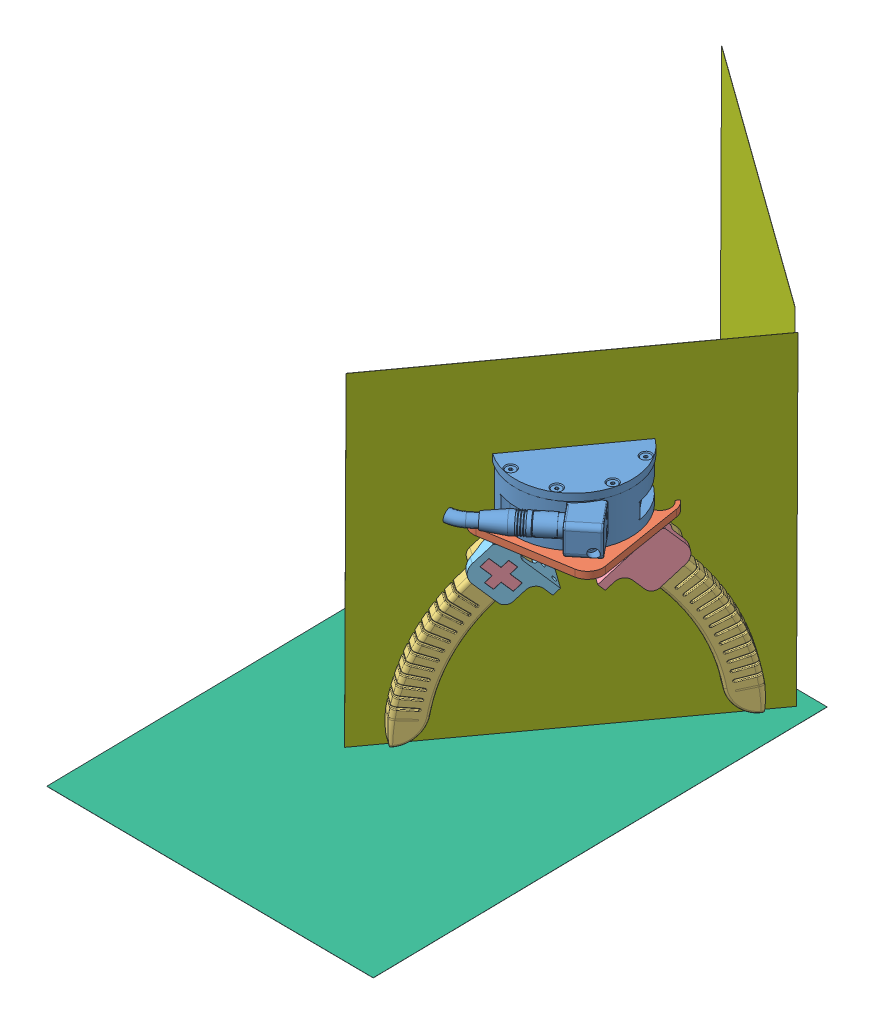
SolidWorks assembly grippper_with_sensor, configuration Default. Lengths in mm.
Overall size (212.48 227.73 417.89).
59 component instances, 34 part files, 24 mates.
Components (placement in the parent):
- ati_gamma_sensor_mount _up-1: ati_gamma_sensor_mount _up [Default] at (-15.434 18.2375 114.8285) size (94 14.49 94) (hidden)
- ati_gamma_sensor_mount _down_L515-1: ati_gamma_sensor_mount _down_L515 [Default] at (-15.434 18.2375 114.8285) x (0 0 1) z (-1 0 0) size (114.18 58 114.18) (hidden)
- ATI-9105-TIF-GAMMA-1: ATI-9105-TIF-GAMMA [Default] at (-15.434 10.2375 114.8285) x (-0.987109 0 0.160048) z (0 1 0) size (81.43 106.62 33.32)
- fixture-1: fixture [Default] at (15.9943 -30.0869 71.2365) x (-0.987109 0 0.160048) z (0 1 0) size (76 76 7.57)
- Assem_soft-1: Assem_soft [Default] at (-95.8769 -63.8673 78.8152) x (0.181198 -0.950797 -0.251303) z (0.811158 0.000013 0.584827) size (139.54 63.23 30.2)
  - finger_proto_4.2-1: finger_proto_4.2 [Default] at (-2.494 64.561 95.5128) size (120.36 42.19 26.68)
  - linkag_3-1: linkag_3 [Default] at (-2.8273 57.773 71.3134) x (0.891388 0.453242 -0.000014) z (0.000014 0.000003 1) size (40.75 42 30.2)
  - linkage_4-1: linkage_4 [Default] at (-2.8273 57.773 71.3134) x (0.891388 0.453242 -0.000014) z (0.000014 0.000003 1) size (40.75 42 15)
- Assem_soft-2: Assem_soft [Default] at (65.1711 -63.8673 150.9587) x (-0.181198 -0.950797 0.251303) z (-0.811158 0.000013 -0.584827) size (139.54 63.23 30.2)
  - finger_proto_4.2-1: finger_proto_4.2 [Default] at (-2.494 64.561 95.5128) size (120.36 42.19 26.68)
  - linkag_3-1: linkag_3 [Default] at (-2.8273 57.773 71.3134) x (0.891388 0.453242 -0.000014) z (0.000014 0.000003 1) size (40.75 42 30.2)
  - linkage_4-1: linkage_4 [Default] at (-2.8273 57.773 71.3134) x (0.891388 0.453242 -0.000014) z (0.000014 0.000003 1) size (40.75 42 15)
- Assem1-1: Assem1 [Default] at (17.137 -120.8618 -18.1601) x (0.539853 0.425322 0.726403) z (-0.534722 0.839751 -0.094291) size (112.36 145.16 142) (hidden)
  - CAM holder (1)-1: CAM holder (1) [Default] at (82.7281 3.9301 79.7737) x (0.895378 -0.021687 -0.444779) z (0.425322 0.33752 0.839751) size (64.99 120.47 90)
  - Top CAM (1)-1: Top CAM (1) [Default] at (81.9279 129.0526 71.921) x (0.895378 -0.021687 -0.444779) z (-0.425322 -0.33752 -0.839751) size (65 111.17 15.1)
- Intel_RealSense_L515_CAD_external.stp-1: Intel_RealSense_L515_CAD_external.stp [Default] at (106.8055 -15.7625 -7.3222) x (-0.587716 0 -0.809067) z (0 -1 0) size (61.01 64.04 35.39) (hidden)
  - TA_PERIPHERAL_L515_ASM_25_ASM.stp-1: TA_PERIPHERAL_L515_ASM_25_ASM.stp [Default] at origin size (61.01 64.04 35.39)
    - CENTER_HEAT_SINK_SUBASM_L515_AS_ASM.stp-1: CENTER_HEAT_SINK_SUBASM_L515_AS_ASM.stp [Default] at origin size (26.06 28.22 15.92)
      - OPTICAL_HEAD_GEN_1_L515_ASM_6_ASM.stp-1: OPTICAL_HEAD_GEN_1_L515_ASM_6_ASM.stp [Default] at origin size (26.06 28.22 15.92)
        - RXFOV_72X60_P_040419_2.stp-1: RXFOV_72X60_P_040419_2.stp [Default] at (-18.5 -15 -9.623) size (26.06 21.31 15.92) (hidden)
        - TX_FOV_1_2_73X59_040419_2.stp-1: TX_FOV_1_2_73X59_040419_2.stp [Default] at (-18.5 -15 -9.623) size (19.97 16.11 9.45) (hidden)
    - FRONT_OPTICAL_ASSEMBLY_L515_ASM_ASM.stp-1: FRONT_OPTICAL_ASSEMBLY_L515_ASM_ASM.stp [Default] at origin size (24.45 11.78 6.27)
      - CAMERA_2MP_FF_OV2740_CMOS_ASM_1_ASM.stp-1: CAMERA_2MP_FF_OV2740_CMOS_ASM_1_ASM.stp [Default] at (0 0 -22.68) size (8 5.7 2.8)
        - L500_RGB_2MP_1_2_2.stp-1: L500_RGB_2MP_1_2_2.stp [Default] at origin size (8 5.7 2.8)
      - PCB_ASSY_RGB_INTERPOSER_L515_AS_ASM.stp-1: PCB_ASSY_RGB_INTERPOSER_L515_AS_ASM.stp [Default] at origin size (24.45 11.78 3.75)
        - RGB_INTERPOSER_AS03021_23AUG_7.stp-1: RGB_INTERPOSER_AS03021_23AUG_7.stp [Default] at (-14.55 7.36 -5.546) size (24.45 11.78 3.72)
        - KAPTON_RGB_INTERPOSER_L515_8.stp-1: KAPTON_RGB_INTERPOSER_L515_8.stp [Default] at origin size (20.84 11.78 0.05)
        - CONN_FPC_BTM_21POS_-3MM_PITCH_2.stp-1: CONN_FPC_BTM_21POS_-3MM_PITCH_2.stp [Default] at (11.985 13.432 -5.615) x (0 -1 0) z (1 0 0) size (7.5 0.9 2.83)
        - CONN_HEADER_3-0MM_20POS_PWR_2.stp-1: CONN_HEADER_3-0MM_20POS_PWR_2.stp [Default] at (-10.26 11.36 -5.58) x (0 -1 0) z (0 0 -1) size (5.9 2.35 2.24)
    - PCB_ASSEMBLY_MA_ASIC_L515_ASM_5_ASM.stp-1: PCB_ASSEMBLY_MA_ASIC_L515_ASM_5_ASM.stp [Default] at origin size (43.47 31.41 6.28)
      - L500_PCB_ASIC_BOARD_OCT08_ASM_1_ASM.stp-1: L500_PCB_ASIC_BOARD_OCT08_ASM_1_ASM.stp [Default] at (0 0 0.6) size (43.47 31.41 6.28)
        - A-PCB_ASIC_20_ASM_1_ASM_1_ASM.stp-1: A-PCB_ASIC_20_ASM_1_ASM_1_ASM.stp [Default] at origin size (43.47 31.41 6.28)
          - 2UB2C02-000111F_3D_USB_TYPE_C_1_ASM.stp-1: 2UB2C02-000111F_3D_USB_TYPE_C_1_ASM.stp [Default] at (-14.4895 -10.5138 -15.4) x (-0.58723 0.80942 0) z (0 0 -1) size (9.7 11.1 6.08)
            - 2UB2C02-000111F_3D_USB_TYPE_C_2.stp-1: 2UB2C02-000111F_3D_USB_TYPE_C_2.stp [Default] at origin size (9.7 11.1 6.08)
            - 2UB2C02-000111F_3D_USB_TYPE_C_3.stp-1: 2UB2C02-000111F_3D_USB_TYPE_C_3.stp [Default] at origin size (0.28 0.35 0.16)
          - P-PCB_ASIC_20_1_3.stp-1: P-PCB_ASIC_20_1_3.stp [Default] at origin size (41.95 30.8 1)
      - BM03B-SRSS-TB_1.stp-1: BM03B-SRSS-TB_1.stp [Default] at (15.2095 -11.0504 -16.2) x (0.587785 0.809017 0) z (0 0 -1) size (5 4.32 3.6)
    - REAR_HOUSING_ASSEMBLY_L515_ASM__ASM.stp-1: REAR_HOUSING_ASSEMBLY_L515_ASM__ASM.stp [Default] at origin size (61.01 64.04 26)
      - INTAKE_VENT_L515_9.stp-1: INTAKE_VENT_L515_9.stp [Default] at origin size (12.82 7.66 16.91)
      - INTAKE_VENT_L515_9.stp-2: INTAKE_VENT_L515_9.stp [Default] x (0.660526 0.750803 0) z (0 0 1) size (12.82 7.66 16.91)
      - REAR_HOUSING_L515_25.stp-1: REAR_HOUSING_L515_25.stp [Default] at origin size (61.01 61.01 26)
    - COVER_WINDOW_SUBASM_L515_ASM_2_ASM.stp-1: COVER_WINDOW_SUBASM_L515_ASM_2_ASM.stp [Default] at origin size (57.86 57.86 2.18)
      - COVER_WINDOW_IR_W_ADHESIVE_L515_ASM.stp-1: COVER_WINDOW_IR_W_ADHESIVE_L515_ASM.stp [Default] at origin size (57.86 57.86 0.78)
        - COVER_WINDOW_IR_L515_10.stp-1: COVER_WINDOW_IR_L515_10.stp [Default] at origin size (57.86 57.86 0.5)
        - COVER_WINDOW_MASK_L515_10.stp-1: COVER_WINDOW_MASK_L515_10.stp [Default] at origin size (57.56 57.56 0.03)
        - COVER_WINDOW_RGB_RING_L515_8.stp-1: COVER_WINDOW_RGB_RING_L515_8.stp [Default] at origin size (7.8 7.8 0.03)
        - ADHESIVE_COVER_WINDOW_IR_L515_1.stp-1: ADHESIVE_COVER_WINDOW_IR_L515_1.stp [Default] at origin size (57.36 57.36 0.25)
      - FOAM_ISOLATION_RGB_L515_ASM_15_ASM.stp-1: FOAM_ISOLATION_RGB_L515_ASM_15_ASM.stp [Default] at origin size (18 37.16 1.6)
        - FOAM_ISOLATION_RGB_L515_13.stp-1: FOAM_ISOLATION_RGB_L515_13.stp [Default] at origin size (18 37.16 1.5)
        - ADHESIVE_ISOLATION_RGB_L515_11.stp-1: ADHESIVE_ISOLATION_RGB_L515_11.stp [Default] at origin size (18 37.16 0.1)
      - COVER_WINDOW_SLOT_FILLER_L515_8.stp-1: COVER_WINDOW_SLOT_FILLER_L515_8.stp [Default] at origin size (15.1 1.1 0.5)
      - FOAM_SEALING_CW_FHS_L515_16.stp-1: FOAM_SEALING_CW_FHS_L515_16.stp [Default] at origin size (39.78 43.86 1.4)
    - AUX_DOOR_ASSEMBLY_L515_ASM_7_ASM.stp-1: AUX_DOOR_ASSEMBLY_L515_ASM_7_ASM.stp [Default] at origin size (9.18 11.47 3.61)
      - AUX_DOOR_L515_8.stp-1: AUX_DOOR_L515_8.stp [Default] at origin size (9.18 11.47 3.61)
      - STEEL_PIN_2.stp-1: STEEL_PIN_2.stp [Default] at (25.6249 -13.3025 -17.25) x (-0.587785 -0.809017 0) z (-0.809017 0.587785 0) size (1.6 1.6 1.6)
      - STEEL_PIN_2.stp-2: STEEL_PIN_2.stp [Default] at (20.57 -20.26 -17.25) x (-0.587785 -0.809017 0) z (-0.809017 0.587785 0) size (1.6 1.6 1.6)
- A4 paper-1: A4 paper [Default] at (57.928 -150.2352 318.2559) x (-0.999818 0.017006 0.008599) z (0.008459 -0.008282 0.99993) size (210 0.1 297)
- frame-1: frame [Default] at (-77.5769 -146.9678 201.3643) x (0.001981 0.999994 -0.002747) z (-0.584817 0.003387 0.811158) size (210 0.1 210)
- frame-2: frame [Default] at (37.8731 -139.7626 25.5573) x (0.001981 0.999994 -0.002747) z (0.811163 0 0.584821) size (210 0.1 210)
Mates (geometry in assembly coordinates):
- Coincident1: coincident anti-aligned: plane of ati_gamma_sensor_mount _up-1 through (-15.434 18.2375 114.8285) normal (0 -1 0); plane of ati_gamma_sensor_mount _down_L515-1 through (-15.434 18.2375 114.8285) normal (0 1 0)
- Coincident4: coincident anti-aligned: plane of ati_gamma_sensor_mount _down_L515-1 through (-15.434 10.2375 114.8285) normal (0 -1 0); plane of ATI-9105-TIF-GAMMA-1 through (-15.434 10.2375 114.8285) normal (0 1 0)
- Coincident8: coincident anti-aligned: plane of ATI-9105-TIF-GAMMA-1 through (-15.434 -23.0869 114.8285) normal (0 -1 0); plane of fixture-1 through (-15.434 -23.0869 114.8285) normal (0 1 0)
- Concentric3: concentric aligned: cylinder of ATI-9105-TIF-GAMMA-1 through (-0.8135 -17.4869 94.5494) axis (0 -1 0) radius 2.5502; cylinder of fixture-1 through (-0.8135 -26.2869 94.5494) axis (0 -1 0) radius 7.25
- Concentric4: concentric anti-aligned: cylinder of ATI-9105-TIF-GAMMA-1 through (-30.0545 -17.4869 135.1075) axis (0 -1 0) radius 2.5502; cylinder of fixture-1 through (-30.0545 -30.0869 135.1075) axis (0 1 0) radius 3.1
- Concentric5: concentric aligned: cylinder of fixture-1 through (-13.83 -30.0869 93.7945) axis (0 1 0) radius 1.575; cylinder of Assem_soft-1/linkage_4-1 through (-13.83 -38.0869 93.7945) axis (0 1 0) radius 1.5
- Concentric6: concentric aligned: cylinder of fixture-1 through (4.1778 -30.0869 106.7775) axis (0 1 0) radius 1.575; cylinder of Assem_soft-1/linkag_3-1 through (4.1778 -38.0869 106.7775) axis (0 1 0) radius 1.5
- Coincident9: coincident anti-aligned: plane of fixture-1 through (15.9943 -30.0869 71.2365) normal (0 -1 0); plane of Assem_soft-1/linkag_3-1 through (-1.991 -30.0869 108.4941) normal (0 1 0)
- Coincident10: coincident anti-aligned: plane of fixture-1 through (15.9943 -30.0869 71.2365) normal (0 -1 0); plane of Assem_soft-2/linkag_3-1 through (-28.7148 -30.0869 121.2799) normal (0 1 0)
- Concentric7: concentric aligned: cylinder of fixture-1 through (-34.8836 -30.0869 122.9964) axis (0 1 0) radius 1.575; cylinder of Assem_soft-2/linkag_3-1 through (-34.8836 -38.0869 122.9964) axis (0 1 0) radius 1.5
- Concentric8: concentric aligned: circle of fixture-1; cylinder of Assem_soft-2/linkage_4-1 through (-16.8758 -38.0869 135.9794) axis (0 1 0) radius 1.5
- Coincident11: coincident anti-aligned: plane of ati_gamma_sensor_mount _down_L515-1 through (51.7411 10.2375 61.7955) normal (0.707107 0 -0.707107); plane of Assem1-1/CAM holder (1)-1 through (21.6891 -17.3593 31.7434) normal (-0.707107 0 0.707107)
- Concentric9: concentric anti-aligned: cylinder of ati_gamma_sensor_mount _down_L515-1 through (39.0132 60.2375 60.3813) axis (0.707107 0 -0.707107) radius 3.05; circle of Assem1-1/CAM holder (1)-1
- Parallel1: parallel anti-aligned: plane of fixture-1 through (15.9943 -30.0869 71.2365) normal (0 -1 0); plane of Intel_RealSense_L515_CAD_external.stp-1/TA_PERIPHERAL_L515_ASM_25_ASM.stp-1/REAR_HOUSING_ASSEMBLY_L515_ASM__ASM.stp-1/REAR_HOUSING_L515_25.stp-1 through (106.8055 10.2375 -7.3222) normal (0 1 0)
- Coincident13: coincident anti-aligned: plane of ati_gamma_sensor_mount _down_L515-1 through (-15.434 10.2375 114.8285) normal (0 -1 0); plane of Intel_RealSense_L515_CAD_external.stp-1/TA_PERIPHERAL_L515_ASM_25_ASM.stp-1/REAR_HOUSING_ASSEMBLY_L515_ASM__ASM.stp-1/REAR_HOUSING_L515_25.stp-1 through (106.8055 10.2375 -7.3222) normal (0 1 0)
- Concentric10: concentric anti-aligned: cylinder of ati_gamma_sensor_mount _down_L515-1 through (39.0132 30.2375 60.3813) axis (0.707107 0 -0.707107) radius 3.05; circle of Assem1-1/CAM holder (1)-1
- Coincident14: coincident aligned: plane of ati_gamma_sensor_mount _up-1 through (31.566 26.2375 67.8285) normal (1 0 0); plane of ati_gamma_sensor_mount _down_L515-1 through (31.566 10.2375 67.8285) normal (1 0 0)
- Concentric11: concentric aligned: cylinder of ati_gamma_sensor_mount _up-1 through (-53.434 18.2375 76.8285) axis (0 1 0) radius 3.1; cylinder of ati_gamma_sensor_mount _down_L515-1 through (-53.434 10.2375 76.8285) axis (0 1 0) radius 3.1
- Concentric13: concentric aligned: cylinder of Assem1-1/Top CAM (1)-1 through (106.8055 14.9375 -7.3222) axis (0 -1 0) radius 9.8; cylinder of Intel_RealSense_L515_CAD_external.stp-1/TA_PERIPHERAL_L515_ASM_25_ASM.stp-1/REAR_HOUSING_ASSEMBLY_L515_ASM__ASM.stp-1/REAR_HOUSING_L515_25.stp-1 through (106.8055 11.5375 -7.3222) axis (0 -1 0) radius 30.5
- Coincident16: coincident anti-aligned: plane of ati_gamma_sensor_mount _down_L515-1 through (-15.434 10.2375 114.8285) normal (0 -1 0); plane of ATI-9105-TIF-GAMMA-1 through (-15.434 10.2375 114.8285) normal (0 1 0)
- Concentric14: concentric anti-aligned: cylinder of ati_gamma_sensor_mount _up-1 through (-15.434 32.6375 114.8285) axis (0 -1 0) radius 40; cylinder of ATI-9105-TIF-GAMMA-1 through (-15.434 5.5131 114.8285) axis (0 1 0) radius 37.719
- Coincident24: coincident anti-aligned: plane of frame-1 through (-77.658 -146.9678 201.3058) normal (-0.811163 0 -0.584821)
- Coincident25: coincident: plane of A4 paper-1 through (57.928 -150.2352 318.2559) normal (0.017076 0.999821 0.008137); line of frame-1 through (45.1537 -147.679 30.9627) axis (-0.584817 0.003387 0.811158)
- Coincident27: coincident anti-aligned: plane of frame-1 through (45.1537 -147.679 30.9627) normal (0.584817 -0.003387 -0.811158); plane of frame-2 through (37.8146 -139.7622 25.6384) normal (-0.584817 0.003387 0.811158)
